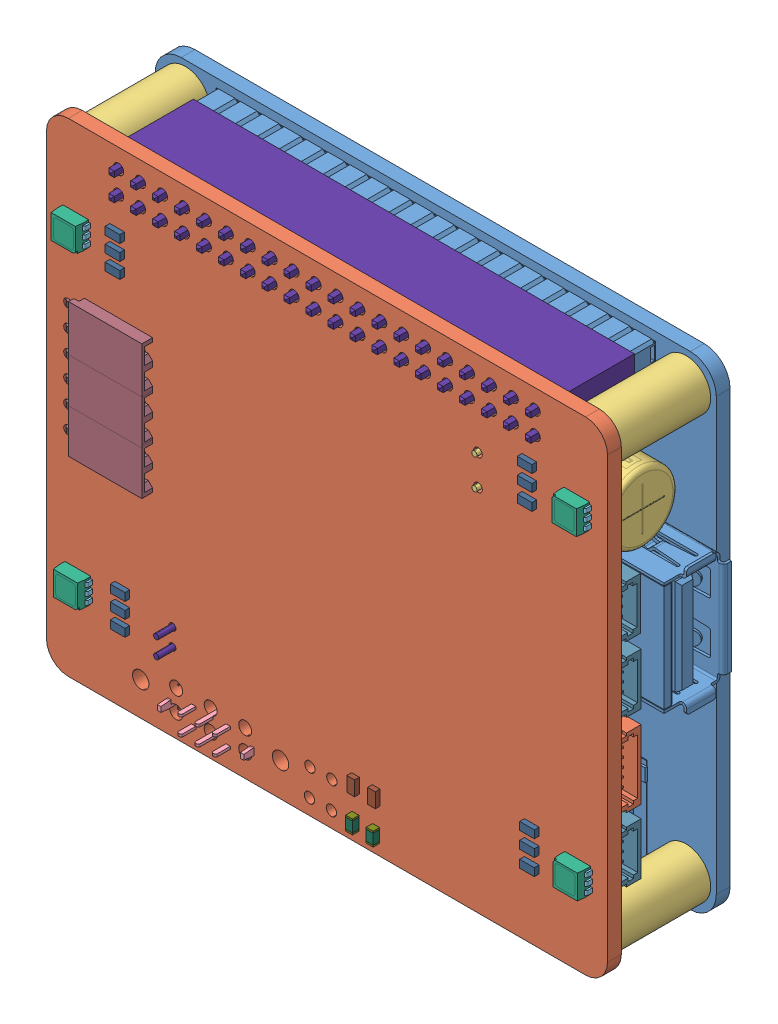
SolidWorks assembly STMf303 hat + RPi 3A+, configuration Default. Lengths in mm.
Overall size (68.17 58.5 17.95).
303 component instances, 40 part files, 5 mates.
Components (placement in the parent):
- Raspberry PI 3 Model A+-1: Raspberry PI 3 Model A+ [Défaut] at (135.3946 10.6154 11.2635) size (68.17 58.5 11.94)
- FC_PiHat_REV1-1: FC_PiHat_REV1 [Default] at (41.2941 -16.4646 23.8635) x (-1 0 0) z (0 0 -1) size (65 56 12.01)
  - FC_PiHat_REV1.step-1: FC_PiHat_REV1.step [Default] at origin size (65 56 12.01)
    - J7FC_PiHat_REV1.step-1: J7FC_PiHat_REV1.step [Default] at origin size (8 4.95 2.96)
      - SM06B-SRSS-TB.step-1: SM06B-SRSS-TB.step [Default] at (13.3 4.6 -0.3) x (1 0 0) z (0 -1 0) size (8 2.96 4.95)
    - C10FC_PiHat_REV1.step-1: C10FC_PiHat_REV1.step [Default] at origin size (13.96 8.06 10.04)
      - User_Library-Cap_electro_8x11_5x3_5mm_RA.step-1: User_Library-Cap_electro_8x11_5x3_5mm_RA.step [Default] at (13.5254 44.5 4) x (0 1 0) z (0 0 1) size (8.06 13.96 10.04)
    - J11FC_PiHat_REV1.step-1: J11FC_PiHat_REV1.step [Default] at origin size (10 6 9.8)
      - User_Library-EG1940-ND.step-1: User_Library-EG1940-ND.step [Default] at (40.9499 0.2249 0) x (1 0 0) z (0 0 1) size (10 6 9.8)
    - D4FC_PiHat_REV1.step-1: D4FC_PiHat_REV1.step [Default] at origin size (3.4 2.8 1.85)
      - User_Library-RGB_LED_Zwart_ASMT-YTC2-0AA02.step-1: User_Library-RGB_LED_Zwart_ASMT-YTC2-0AA02.step [Default] at (2.2908 8.9737 -1.6023) x (-1 0 0) z (0 -1 0) size (3.4 1.85 2.8)
        - Pootje_RGB_LED.step-1: Pootje_RGB_LED.step [Default] at (-0.3594 -0.1975 0.3238) size (0.9 1.1 0.5)
        - ASMT-YTC2-0AA02.step-1: ASMT-YTC2-0AA02.step [Default] at (-2.6594 -0.3475 0.5738) size (3 1.8 2.8)
        - Pootje_RGB_LED.step-2: Pootje_RGB_LED.step [Default] at (-0.3594 -0.1975 -0.5762) size (0.9 1.1 0.5)
        - Pootje_RGB_LED.step-3: Pootje_RGB_LED.step [Default] at (-0.3594 -0.1975 -1.4762) size (0.9 1.1 0.5)
        - Pootje_RGB_LED.step-4: Pootje_RGB_LED.step [Default] at (-1.9594 -0.1975 -1.9762) x (-1 0 0) z (0 0 -1) size (0.9 1.1 0.5)
        - Pootje_RGB_LED.step-5: Pootje_RGB_LED.step [Default] at (-1.9594 -0.1975 -1.0762) x (-1 0 0) z (0 0 -1) size (0.9 1.1 0.5)
        - Pootje_RGB_LED.step-6: Pootje_RGB_LED.step [Default] at (-1.9594 -0.1975 -0.1762) x (-1 0 0) z (0 0 -1) size (0.9 1.1 0.5)
    - D3FC_PiHat_REV1.step-1: D3FC_PiHat_REV1.step [Default] at origin size (3.4 2.8 1.85)
      - User_Library-RGB_LED_Zwart_ASMT-YTC2-0AA02.step-1: User_Library-RGB_LED_Zwart_ASMT-YTC2-0AA02.step [Default] at (2.3908 45.4737 -1.6023) x (-1 0 0) z (0 -1 0) size (3.4 1.85 2.8)
        - Pootje_RGB_LED.step-1: Pootje_RGB_LED.step [Default] at (-0.3594 -0.1975 0.3238) size (0.9 1.1 0.5)
        - ASMT-YTC2-0AA02.step-1: ASMT-YTC2-0AA02.step [Default] at (-2.6594 -0.3475 0.5738) size (3 1.8 2.8)
        - Pootje_RGB_LED.step-2: Pootje_RGB_LED.step [Default] at (-0.3594 -0.1975 -0.5762) size (0.9 1.1 0.5)
        - Pootje_RGB_LED.step-3: Pootje_RGB_LED.step [Default] at (-0.3594 -0.1975 -1.4762) size (0.9 1.1 0.5)
        - Pootje_RGB_LED.step-4: Pootje_RGB_LED.step [Default] at (-1.9594 -0.1975 -1.9762) x (-1 0 0) z (0 0 -1) size (0.9 1.1 0.5)
        - Pootje_RGB_LED.step-5: Pootje_RGB_LED.step [Default] at (-1.9594 -0.1975 -1.0762) x (-1 0 0) z (0 0 -1) size (0.9 1.1 0.5)
        - Pootje_RGB_LED.step-6: Pootje_RGB_LED.step [Default] at (-1.9594 -0.1975 -0.1762) x (-1 0 0) z (0 0 -1) size (0.9 1.1 0.5)
    - D2FC_PiHat_REV1.step-1: D2FC_PiHat_REV1.step [Default] at origin size (3.4 2.8 1.85)
      - User_Library-RGB_LED_Zwart_ASMT-YTC2-0AA02.step-1: User_Library-RGB_LED_Zwart_ASMT-YTC2-0AA02.step [Default] at (62.5092 10.7763 -1.6023) x (1 0 0) z (0 1 0) size (3.4 1.85 2.8)
        - Pootje_RGB_LED.step-1: Pootje_RGB_LED.step [Default] at (-0.3594 -0.1975 0.3238) size (0.9 1.1 0.5)
        - ASMT-YTC2-0AA02.step-1: ASMT-YTC2-0AA02.step [Default] at (-2.6594 -0.3475 0.5738) size (3 1.8 2.8)
        - Pootje_RGB_LED.step-2: Pootje_RGB_LED.step [Default] at (-0.3594 -0.1975 -0.5762) size (0.9 1.1 0.5)
        - Pootje_RGB_LED.step-3: Pootje_RGB_LED.step [Default] at (-0.3594 -0.1975 -1.4762) size (0.9 1.1 0.5)
        - Pootje_RGB_LED.step-4: Pootje_RGB_LED.step [Default] at (-1.9594 -0.1975 -1.9762) x (-1 0 0) z (0 0 -1) size (0.9 1.1 0.5)
        - Pootje_RGB_LED.step-5: Pootje_RGB_LED.step [Default] at (-1.9594 -0.1975 -1.0762) x (-1 0 0) z (0 0 -1) size (0.9 1.1 0.5)
        - Pootje_RGB_LED.step-6: Pootje_RGB_LED.step [Default] at (-1.9594 -0.1975 -0.1762) x (-1 0 0) z (0 0 -1) size (0.9 1.1 0.5)
    - D1FC_PiHat_REV1.step-1: D1FC_PiHat_REV1.step [Default] at origin size (3.4 2.8 1.85)
      - User_Library-RGB_LED_Zwart_ASMT-YTC2-0AA02.step-1: User_Library-RGB_LED_Zwart_ASMT-YTC2-0AA02.step [Default] at (62.7592 46.4263 -1.6023) x (1 0 0) z (0 1 0) size (3.4 1.85 2.8)
        - Pootje_RGB_LED.step-1: Pootje_RGB_LED.step [Default] at (-0.3594 -0.1975 0.3238) size (0.9 1.1 0.5)
        - ASMT-YTC2-0AA02.step-1: ASMT-YTC2-0AA02.step [Default] at (-2.6594 -0.3475 0.5738) size (3 1.8 2.8)
        - Pootje_RGB_LED.step-2: Pootje_RGB_LED.step [Default] at (-0.3594 -0.1975 -0.5762) size (0.9 1.1 0.5)
        - Pootje_RGB_LED.step-3: Pootje_RGB_LED.step [Default] at (-0.3594 -0.1975 -1.4762) size (0.9 1.1 0.5)
        - Pootje_RGB_LED.step-4: Pootje_RGB_LED.step [Default] at (-1.9594 -0.1975 -1.9762) x (-1 0 0) z (0 0 -1) size (0.9 1.1 0.5)
        - Pootje_RGB_LED.step-5: Pootje_RGB_LED.step [Default] at (-1.9594 -0.1975 -1.0762) x (-1 0 0) z (0 0 -1) size (0.9 1.1 0.5)
        - Pootje_RGB_LED.step-6: Pootje_RGB_LED.step [Default] at (-1.9594 -0.1975 -0.1762) x (-1 0 0) z (0 0 -1) size (0.9 1.1 0.5)
    - S1FC_PiHat_REV1.step-1: S1FC_PiHat_REV1.step [Default] at origin size (4.1 4.1 0.81)
      - 5843174976.step-1: 5843174976.step [Default] at (40.7 32.3 0) size (4.1 4.1 0.81)
        - Body.step-1: Body.step [Default] at (-2.05 -2.05 0)
          - Open_CASCADE_STEP_translator_6.8_14.2.1.x_t-1: Open_CASCADE_STEP_translator_6.8_14.2.1.x_t [Default] at origin
        - Open_CASCADE_STEP_translator_6.8_14.1.step-1: Open_CASCADE_STEP_translator_6.8_14.1.step [Default] at (-2.05 -2.05 0) size (0.52 0.52 0.01)
        - Thermal_Shape.step-1: Thermal_Shape.step [Default] at (-1.3 -1.35 -0.001) size (2.6 2.7 0)
        - Pin_Shape.step-1: Pin_Shape.step [Default] at (-2.05 -1.37 0) size (0.35 0.24 0)
        - Pin_Shape.step-2: Pin_Shape.step [Default] at (2.05 1.37 0) x (-1 0 0) z (0 0 1) size (0.35 0.24 0)
        - Pin_Shape.step-3: Pin_Shape.step [Default] at (-2.05 -0.87 0) size (0.35 0.24 0)
        - Pin_Shape.step-4: Pin_Shape.step [Default] at (2.05 0.87 0) x (-1 0 0) z (0 0 1) size (0.35 0.24 0)
        - Pin_Shape.step-5: Pin_Shape.step [Default] at (-2.05 -0.37 0) size (0.35 0.24 0)
        - Pin_Shape.step-6: Pin_Shape.step [Default] at (2.05 0.37 0) x (-1 0 0) z (0 0 1) size (0.35 0.24 0)
        - Pin_Shape.step-7: Pin_Shape.step [Default] at (-2.05 0.13 0) size (0.35 0.24 0)
        - Pin_Shape.step-8: Pin_Shape.step [Default] at (2.05 -0.13 0) x (-1 0 0) z (0 0 1) size (0.35 0.24 0)
        - Pin_Shape.step-9: Pin_Shape.step [Default] at (-2.05 0.63 0) size (0.35 0.24 0)
        - Pin_Shape.step-10: Pin_Shape.step [Default] at (2.05 -0.63 0) x (-1 0 0) z (0 0 1) size (0.35 0.24 0)
        - Pin_Shape.step-11: Pin_Shape.step [Default] at (-2.05 1.13 0) size (0.35 0.24 0)
        - Pin_Shape.step-12: Pin_Shape.step [Default] at (2.05 -1.13 0) x (-1 0 0) z (0 0 1) size (0.35 0.24 0)
        - Pin_Shape.step-13: Pin_Shape.step [Default] at (-1.13 -2.05 0) x (0 1 0) z (0 0 1) size (0.35 0.24 0)
        - Pin_Shape.step-14: Pin_Shape.step [Default] at (1.13 2.05 0) x (0 -1 0) z (0 0 1) size (0.35 0.24 0)
        - Pin_Shape.step-15: Pin_Shape.step [Default] at (-0.63 -2.05 0) x (0 1 0) z (0 0 1) size (0.35 0.24 0)
        - Pin_Shape.step-16: Pin_Shape.step [Default] at (0.63 2.05 0) x (0 -1 0) z (0 0 1) size (0.35 0.24 0)
        - Pin_Shape.step-17: Pin_Shape.step [Default] at (-0.13 -2.05 0) x (0 1 0) z (0 0 1) size (0.35 0.24 0)
        - Pin_Shape.step-18: Pin_Shape.step [Default] at (0.13 2.05 0) x (0 -1 0) z (0 0 1) size (0.35 0.24 0)
        - Pin_Shape.step-19: Pin_Shape.step [Default] at (0.37 -2.05 0) x (0 1 0) z (0 0 1) size (0.35 0.24 0)
        - Pin_Shape.step-20: Pin_Shape.step [Default] at (-0.37 2.05 0) x (0 -1 0) z (0 0 1) size (0.35 0.24 0)
        - Pin_Shape.step-21: Pin_Shape.step [Default] at (0.87 -2.05 0) x (0 1 0) z (0 0 1) size (0.35 0.24 0)
        - Pin_Shape.step-22: Pin_Shape.step [Default] at (-0.87 2.05 0) x (0 -1 0) z (0 0 1) size (0.35 0.24 0)
        - Pin_Shape.step-23: Pin_Shape.step [Default] at (1.37 -2.05 0) x (0 1 0) z (0 0 1) size (0.35 0.24 0)
        - Pin_Shape.step-24: Pin_Shape.step [Default] at (-1.37 2.05 0) x (0 -1 0) z (0 0 1) size (0.35 0.24 0)
    - R14FC_PiHat_REV1.step-1: R14FC_PiHat_REV1.step [Default] at origin size (1.7 0.9 0.55)
      - 6063442624.step-1: 6063442624.step [Default] at (8.7742 7.9 -2.1523) size (1.7 0.9 0.55)
        - Extruded.step-1: Extruded.step [Default] at origin size (1.7 0.9 0.55)
    - R13FC_PiHat_REV1.step-1: R13FC_PiHat_REV1.step [Default] at origin size (1.7 0.9 0.55)
      - 6063442624.step-1: 6063442624.step [Default] at (8.7742 9.8048 -2.1523) size (1.7 0.9 0.55)
        - Extruded.step-1: Extruded.step [Default] at origin size (1.7 0.9 0.55)
    - R12FC_PiHat_REV1.step-1: R12FC_PiHat_REV1.step [Default] at origin size (1.7 0.9 0.55)
      - 6063442624.step-1: 6063442624.step [Default] at (8.7742 11.7 -2.1523) size (1.7 0.9 0.55)
        - Extruded.step-1: Extruded.step [Default] at origin size (1.7 0.9 0.55)
    - R11FC_PiHat_REV1.step-1: R11FC_PiHat_REV1.step [Default] at origin size (1.7 0.9 0.55)
      - 6063442624.step-1: 6063442624.step [Default] at (9.05 44.4 -2.1523) size (1.7 0.9 0.55)
        - Extruded.step-1: Extruded.step [Default] at origin size (1.7 0.9 0.55)
    - R10FC_PiHat_REV1.step-1: R10FC_PiHat_REV1.step [Default] at origin size (1.7 0.9 0.55)
      - 6063442624.step-1: 6063442624.step [Default] at (9.05 46.3 -2.1523) size (1.7 0.9 0.55)
        - Extruded.step-1: Extruded.step [Default] at origin size (1.7 0.9 0.55)
    - R9FC_PiHat_REV1.step-1: R9FC_PiHat_REV1.step [Default] at origin size (0.9 1.7 0.55)
      - 6063442432.step-1: 6063442432.step [Default] at (59.9 29.7 0) size (0.9 1.7 0.55)
        - Extruded-0.step-1: Extruded-0.step [Default] at origin size (0.9 1.7 0.55)
    - R8FC_PiHat_REV1.step-1: R8FC_PiHat_REV1.step [Default] at origin size (1.7 0.9 0.55)
      - 6063442624.step-1: 6063442624.step [Default] at (9.05 48.2 -2.1523) size (1.7 0.9 0.55)
        - Extruded.step-1: Extruded.step [Default] at origin size (1.7 0.9 0.55)
    - R7FC_PiHat_REV1.step-1: R7FC_PiHat_REV1.step [Default] at origin size (1.84 1.84 0.55)
      - 6063441088.step-1: 6063441088.step [Default] at (39.9 37.9 0) size (1.84 1.84 0.55)
        - Extruded-1.step-1: Extruded-1.step [Default] at origin size (1.84 1.84 0.55)
    - R6FC_PiHat_REV1.step-1: R6FC_PiHat_REV1.step [Default] at origin size (1.7 0.9 0.55)
      - 6063442624.step-1: 6063442624.step [Default] at (56.2 11.8 -2.1523) size (1.7 0.9 0.55)
        - Extruded.step-1: Extruded.step [Default] at origin size (1.7 0.9 0.55)
    - R5FC_PiHat_REV1.step-1: R5FC_PiHat_REV1.step [Default] at origin size (1.7 0.9 0.55)
      - 6063442624.step-1: 6063442624.step [Default] at (56.2 10 -2.1523) size (1.7 0.9 0.55)
        - Extruded.step-1: Extruded.step [Default] at origin size (1.7 0.9 0.55)
    - R4FC_PiHat_REV1.step-1: R4FC_PiHat_REV1.step [Default] at origin size (1.7 0.9 0.55)
      - 6063442624.step-1: 6063442624.step [Default] at (56.2 8.2 -2.1523) size (1.7 0.9 0.55)
        - Extruded.step-1: Extruded.step [Default] at origin size (1.7 0.9 0.55)
    - R3FC_PiHat_REV1.step-1: R3FC_PiHat_REV1.step [Default] at origin size (1.7 0.9 0.55)
      - 6063442624.step-1: 6063442624.step [Default] at (56.8 47.4 -2.1523) size (1.7 0.9 0.55)
        - Extruded.step-1: Extruded.step [Default] at origin size (1.7 0.9 0.55)
    - R2FC_PiHat_REV1.step-1: R2FC_PiHat_REV1.step [Default] at origin size (1.7 0.9 0.55)
      - 6063442624.step-1: 6063442624.step [Default] at (56.8 45.6 -2.1523) size (1.7 0.9 0.55)
        - Extruded.step-1: Extruded.step [Default] at origin size (1.7 0.9 0.55)
    - R1FC_PiHat_REV1.step-1: R1FC_PiHat_REV1.step [Default] at origin size (1.7 0.9 0.55)
      - 6063442624.step-1: 6063442624.step [Default] at (56.8 43.8 -2.1523) size (1.7 0.9 0.55)
        - Extruded.step-1: Extruded.step [Default] at origin size (1.7 0.9 0.55)
    - J8FC_PiHat_REV1.step-1: J8FC_PiHat_REV1.step [Default] at origin size (4.95 8 2.96)
      - SM06B-SRSS-TB.step-1: SM06B-SRSS-TB.step [Default] at (4.55 19.8 -0.3) x (0 -1 0) z (-1 0 0) size (8 2.96 4.95)
    - J6FC_PiHat_REV1.step-1: J6FC_PiHat_REV1.step [Default] at origin size (10.06 15.53 5.7)
      - female_header_a-bl254-ea-g02d.step-1: female_header_a-bl254-ea-g02d.step [Default] at (61.2001 31.0851 -1.6023) x (0 -1 0) z (0 0 -1) size (5.33 10.06 5.7)
      - female_header_a-bl254-ea-g02d.step-2: female_header_a-bl254-ea-g02d.step [Default] at (61.2001 26.0099 -1.6023) x (0 -1 0) z (0 0 -1) size (5.33 10.06 5.7)
      - female_header_a-bl254-ea-g02d.step-3: female_header_a-bl254-ea-g02d.step [Default] at (61.2001 36.2099 -1.6023) x (0 -1 0) z (0 0 -1) size (5.33 10.06 5.7)
    - J4FC_PiHat_REV1.step-1: J4FC_PiHat_REV1.step [Default] at origin size (4.95 6 2.96)
      - SM04B-SRSS-TB.step-1: SM04B-SRSS-TB.step [Default] at (4.55 28.375 -0.3) x (0 -1 0) z (-1 0 0) size (6 2.96 4.95)
    - J3FC_PiHat_REV1.step-1: J3FC_PiHat_REV1.step [Default] at origin size (4.95 6 2.96)
      - SM04B-SRSS-TB.step-1: SM04B-SRSS-TB.step [Default] at (4.55 11.35 -0.3) x (0 -1 0) z (-1 0 0) size (6 2.96 4.95)
    - J2FC_PiHat_REV1.step-1: J2FC_PiHat_REV1.step [Default] at origin size (8 4.95 2.96)
      - SM06B-SRSS-TB.step-1: SM06B-SRSS-TB.step [Default] at (22.8093 4.575 -0.3) x (1 0 0) z (0 -1 0) size (8 2.96 4.95)
    - J1FC_PiHat_REV1.step-1: J1FC_PiHat_REV1.step [Default] at origin size (4.95 6 2.96)
      - SM04B-SRSS-TB.step-1: SM04B-SRSS-TB.step [Default] at (4.625 35.925 -0.3) x (0 -1 0) z (-1 0 0) size (6 2.96 4.95)
    - C4FC_PiHat_REV1.step-1: C4FC_PiHat_REV1.step [Default] at origin size (0.9 1.8 0.9)
      - 6063440896.step-1: 6063440896.step [Default] at (41.3 27.825 0) size (0.9 1.8 0.9)
        - Extruded-2.step-1: Extruded-2.step [Default] at origin size (0.9 1.8 0.9)
    - C3FC_PiHat_REV1.step-1: C3FC_PiHat_REV1.step [Default] at origin size (0.9 1.8 0.9)
      - 6063440896.step-1: 6063440896.step [Default] at (44.1 32.225 0) size (0.9 1.8 0.9)
        - Extruded-2.step-1: Extruded-2.step [Default] at origin size (0.9 1.8 0.9)
    - C2FC_PiHat_REV1.step-1: C2FC_PiHat_REV1.step [Default] at origin size (1.8 0.9 0.9)
      - 6063441280.step-1: 6063441280.step [Default] at (38.125 28.8 0) size (1.8 0.9 0.9)
        - Extruded-3.step-1: Extruded-3.step [Default] at origin size (1.8 0.9 0.9)
    - C1FC_PiHat_REV1.step-1: C1FC_PiHat_REV1.step [Default] at origin size (1.8 0.9 0.9)
      - 6063441280.step-1: 6063441280.step [Default] at (38.125 26.7 0) size (1.8 0.9 0.9)
        - Extruded-3.step-1: Extruded-3.step [Default] at origin size (1.8 0.9 0.9)
    - J5FC_PiHat_REV1.step-1: J5FC_PiHat_REV1.step [Default] at origin size (51.1 5 11.1)
      - User_Library-Header_2x20_2_54mm.step-1: User_Library-Header_2x20_2_54mm.step [Default] at (56.6601 52.5601 0) x (1 0 0) z (0 -1 0) size (51.1 11.1 5)
    - L2FC_PiHat_REV1.step-1: L2FC_PiHat_REV1.step [Default] at origin size (12.5 12.7 6.1)
      - 5843174592.step-1: 5843174592.step [Default] at (40.7 17.6 0) x (0 1 0) z (0 0 1) size (12.7 12.5 6.1)
        - pin.step-1: pin.step [Default] at (6.35 2.8 0) x (-1 0 0) z (0 0 1) size (4.5 5.6 3)
          - Open_CASCADE_STEP_translator_6.8_3.3.1.step-1: Open_CASCADE_STEP_translator_6.8_3.3.1.step [Default] at origin size (4.5 5.6 3)
        - pin.step-2: pin.step [Default] at (-6.35 -2.8 0) size (4.5 5.6 3)
          - Open_CASCADE_STEP_translator_6.8_3.3.1.step-1: Open_CASCADE_STEP_translator_6.8_3.3.1.step [Default] at origin size (4.5 5.6 3)
        - Body.step-1: Body.step [Default] at (0 0 0.1)
          - Open_CASCADE_STEP_translator_6.8_14.2.1.x_t-1: Open_CASCADE_STEP_translator_6.8_14.2.1.x_t [Default] at origin
        - cylinder.step-1: cylinder.step [Default] at (0 0 0.1) size (12.5 12.5 3)
    - U3FC_PiHat_REV1.step-1: U3FC_PiHat_REV1.step [Default] at origin size (10.3 15.24 4.47)
      - 5843175168.step-1: 5843175168.step [Default] at (52.775 32.425 0) x (0 1 0) z (0 0 1) size (15.24 10.3 4.47)
        - Body-1.step-1: Body-1.step [Default] at (-4.575 -5.15 0) size (9.15 10.3 4.47)
          - Open_CASCADE_STEP_translator_6.8_42.2.1.step-1: Open_CASCADE_STEP_translator_6.8_42.2.1.step [Default] at origin size (9.15 10.3 4.47)
        - tab.step-1: tab.step [Default] at (-4.575 -5.15 0) size (9 10.25 0.35)
          - Open_CASCADE_STEP_translator_6.8_42.8.1.step-1: Open_CASCADE_STEP_translator_6.8_42.8.1.step [Default] at origin size (9 10.25 0.35)
        - Open_CASCADE_STEP_translator_6.8_42.1.step-1: Open_CASCADE_STEP_translator_6.8_42.1.step [Default] at (-4.575 -5.15 0) size (1.3 1.3 0.01)
        - Lead.step-1: Lead.step [Default] at (-4.575 -3.4 0) x (-1 0 0) z (0 0 1) size (5.46 0.75 2.33)
        - Lead.step-2: Lead.step [Default] at (-4.575 -1.7 0) x (-1 0 0) z (0 0 1) size (5.46 0.75 2.33)
        - Lead.step-3: Lead.step [Default] at (-4.575 0 0) x (-1 0 0) z (0 0 1) size (5.46 0.75 2.33)
        - Lead.step-4: Lead.step [Default] at (-4.575 1.7 0) x (-1 0 0) z (0 0 1) size (5.46 0.75 2.33)
        - Lead.step-5: Lead.step [Default] at (-4.575 3.4 0) x (-1 0 0) z (0 0 1) size (5.46 0.75 2.33)
      - 5843175168-4.step-1: 5843175168-4.step [Default] at (52.775 32.425 0) x (0 1 0) z (0 0 1) size (2.73 0.75 0.2)
    - D6FC_PiHat_REV1.step-1: D6FC_PiHat_REV1.step [Default] at origin size (7.55 6.23 2.62)
      - 5843175552.step-1: 5843175552.step [Default] at (51.8001 16.8001 0) x (1 0 0) z (0 0 1) size (7.55 6.22 2.62)
        - Body-2.step-1: Body-2.step [Default] at (-3.555 -3.11 0.25) size (7.12 6.22 2.47)
          - Open_CASCADE_STEP_translator_6.8_45.1.1.step-1: Open_CASCADE_STEP_translator_6.8_45.1.1.step [Default] at origin size (7.12 6.22 2.47)
        - Lead-5.step-1: Lead-5.step [Default] at (2.635 0 0) size (1.14 3 1.53)
        - Lead-5.step-2: Lead-5.step [Default] at (-2.635 0 0) x (-1 0 0) z (0 0 1) size (1.14 3 1.53)
    - U2FC_PiHat_REV1.step-1: U2FC_PiHat_REV1.step [Default] at origin size (3.98 3.97 1)
      - 5843176128.step-1: 5843176128.step [Default] at (49.3313 45.4354 0) x (0.707107 -0.707107 0) z (0 0 1) size (2.8 2.91 1)
        - Body-3.step-1: Body-3.step [Default] at (-0.8 -1.45 0) size (1.6 2.91 0.95)
          - Open_CASCADE_STEP_translator_6.8_3.1.1.step-1: Open_CASCADE_STEP_translator_6.8_3.1.1.step [Default] at origin size (1.6 2.91 0.95)
        - Leader.step-1: Leader.step [Default] at (-0.8 -0.95 0) x (-1 0 0) z (0 0 1) size (0.6 0.5 0.57)
        - Leader.step-2: Leader.step [Default] at (-0.8 0 0) x (-1 0 0) z (0 0 1) size (0.6 0.5 0.57)
        - Leader.step-3: Leader.step [Default] at (-0.8 0.95 0) x (-1 0 0) z (0 0 1) size (0.6 0.5 0.57)
        - Leader.step-4: Leader.step [Default] at (0.8 -0.95 0) size (0.6 0.5 0.57)
        - Leader.step-5: Leader.step [Default] at (0.8 0.95 0) size (0.6 0.5 0.57)
    - U1FC_PiHat_REV1.step-1: U1FC_PiHat_REV1.step [Default] at origin size (18.98 19.05 1.5)
      - 5843174208.step-1: 5843174208.step [Default] at (26.375 36.65 0) x (-0.707107 -0.707107 0) z (0 0 1) size (14.7 14.7 1.5)
        - Body-4.step-1: Body-4.step [Default] at (-5 -5 0) size (10 10 1.5)
          - Open_CASCADE_STEP_translator_6.8_6.1.1.step-1: Open_CASCADE_STEP_translator_6.8_6.1.1.step [Default] at origin size (10 10 1.5)
        - Leader-6.step-1: Leader-6.step [Default] at (-5 -3.75 0) x (-1 0 0) z (0 0 1) size (2.35 0.27 0.85)
        - Leader-6.step-2: Leader-6.step [Default] at (-3.75 5 0) x (0 1 0) z (0 0 1) size (2.35 0.27 0.85)
        - Leader-6.step-3: Leader-6.step [Default] at (5 -3.75 0) size (2.35 0.27 0.85)
        - Leader-6.step-4: Leader-6.step [Default] at (-3.75 -5 0) x (0 -1 0) z (0 0 1) size (2.35 0.27 0.85)
        - Leader-6.step-5: Leader-6.step [Default] at (-5 -3.25 0) x (-1 0 0) z (0 0 1) size (2.35 0.27 0.85)
        - Leader-6.step-6: Leader-6.step [Default] at (-3.25 5 0) x (0 1 0) z (0 0 1) size (2.35 0.27 0.85)
        - Leader-6.step-7: Leader-6.step [Default] at (5 -3.25 0) size (2.35 0.27 0.85)
        - Leader-6.step-8: Leader-6.step [Default] at (-3.25 -5 0) x (0 -1 0) z (0 0 1) size (2.35 0.27 0.85)
        - Leader-6.step-9: Leader-6.step [Default] at (-5 -2.75 0) x (-1 0 0) z (0 0 1) size (2.35 0.27 0.85)
        - Leader-6.step-10: Leader-6.step [Default] at (-2.75 5 0) x (0 1 0) z (0 0 1) size (2.35 0.27 0.85)
        - Leader-6.step-11: Leader-6.step [Default] at (5 -2.75 0) size (2.35 0.27 0.85)
        - Leader-6.step-12: Leader-6.step [Default] at (-2.75 -5 0) x (0 -1 0) z (0 0 1) size (2.35 0.27 0.85)
        - Leader-6.step-13: Leader-6.step [Default] at (-5 -2.25 0) x (-1 0 0) z (0 0 1) size (2.35 0.27 0.85)
        - Leader-6.step-14: Leader-6.step [Default] at (-2.25 5 0) x (0 1 0) z (0 0 1) size (2.35 0.27 0.85)
        - Leader-6.step-15: Leader-6.step [Default] at (5 -2.25 0) size (2.35 0.27 0.85)
        - Leader-6.step-16: Leader-6.step [Default] at (-2.25 -5 0) x (0 -1 0) z (0 0 1) size (2.35 0.27 0.85)
        - Leader-6.step-17: Leader-6.step [Default] at (-5 -1.75 0) x (-1 0 0) z (0 0 1) size (2.35 0.27 0.85)
        - Leader-6.step-18: Leader-6.step [Default] at (-1.75 5 0) x (0 1 0) z (0 0 1) size (2.35 0.27 0.85)
        - Leader-6.step-19: Leader-6.step [Default] at (5 -1.75 0) size (2.35 0.27 0.85)
        - Leader-6.step-20: Leader-6.step [Default] at (-1.75 -5 0) x (0 -1 0) z (0 0 1) size (2.35 0.27 0.85)
        - Leader-6.step-21: Leader-6.step [Default] at (-5 -1.25 0) x (-1 0 0) z (0 0 1) size (2.35 0.27 0.85)
        - Leader-6.step-22: Leader-6.step [Default] at (-1.25 5 0) x (0 1 0) z (0 0 1) size (2.35 0.27 0.85)
        - Leader-6.step-23: Leader-6.step [Default] at (5 -1.25 0) size (2.35 0.27 0.85)
        - Leader-6.step-24: Leader-6.step [Default] at (-1.25 -5 0) x (0 -1 0) z (0 0 1) size (2.35 0.27 0.85)
        - Leader-6.step-25: Leader-6.step [Default] at (-5 -0.75 0) x (-1 0 0) z (0 0 1) size (2.35 0.27 0.85)
        - Leader-6.step-26: Leader-6.step [Default] at (-0.75 5 0) x (0 1 0) z (0 0 1) size (2.35 0.27 0.85)
        - Leader-6.step-27: Leader-6.step [Default] at (5 -0.75 0) size (2.35 0.27 0.85)
        - Leader-6.step-28: Leader-6.step [Default] at (-0.75 -5 0) x (0 -1 0) z (0 0 1) size (2.35 0.27 0.85)
        - Leader-6.step-29: Leader-6.step [Default] at (-5 -0.25 0) x (-1 0 0) z (0 0 1) size (2.35 0.27 0.85)
        - Leader-6.step-30: Leader-6.step [Default] at (-0.25 5 0) x (0 1 0) z (0 0 1) size (2.35 0.27 0.85)
        - Leader-6.step-31: Leader-6.step [Default] at (5 -0.25 0) size (2.35 0.27 0.85)
        - Leader-6.step-32: Leader-6.step [Default] at (-0.25 -5 0) x (0 -1 0) z (0 0 1) size (2.35 0.27 0.85)
        - Leader-6.step-33: Leader-6.step [Default] at (-5 0.25 0) x (-1 0 0) z (0 0 1) size (2.35 0.27 0.85)
        - Leader-6.step-34: Leader-6.step [Default] at (0.25 5 0) x (0 1 0) z (0 0 1) size (2.35 0.27 0.85)
        - Leader-6.step-35: Leader-6.step [Default] at (5 0.25 0) size (2.35 0.27 0.85)
        - Leader-6.step-36: Leader-6.step [Default] at (0.25 -5 0) x (0 -1 0) z (0 0 1) size (2.35 0.27 0.85)
        - Leader-6.step-37: Leader-6.step [Default] at (-5 0.75 0) x (-1 0 0) z (0 0 1) size (2.35 0.27 0.85)
        - Leader-6.step-38: Leader-6.step [Default] at (0.75 5 0) x (0 1 0) z (0 0 1) size (2.35 0.27 0.85)
        - Leader-6.step-39: Leader-6.step [Default] at (5 0.75 0) size (2.35 0.27 0.85)
        - Leader-6.step-40: Leader-6.step [Default] at (0.75 -5 0) x (0 -1 0) z (0 0 1) size (2.35 0.27 0.85)
        - Leader-6.step-41: Leader-6.step [Default] at (-5 1.25 0) x (-1 0 0) z (0 0 1) size (2.35 0.27 0.85)
        - Leader-6.step-42: Leader-6.step [Default] at (1.25 5 0) x (0 1 0) z (0 0 1) size (2.35 0.27 0.85)
        - Leader-6.step-43: Leader-6.step [Default] at (5 1.25 0) size (2.35 0.27 0.85)
        - Leader-6.step-44: Leader-6.step [Default] at (1.25 -5 0) x (0 -1 0) z (0 0 1) size (2.35 0.27 0.85)
        - Leader-6.step-45: Leader-6.step [Default] at (-5 1.75 0) x (-1 0 0) z (0 0 1) size (2.35 0.27 0.85)
        - Leader-6.step-46: Leader-6.step [Default] at (1.75 5 0) x (0 1 0) z (0 0 1) size (2.35 0.27 0.85)
        - Leader-6.step-47: Leader-6.step [Default] at (5 1.75 0) size (2.35 0.27 0.85)
        - Leader-6.step-48: Leader-6.step [Default] at (1.75 -5 0) x (0 -1 0) z (0 0 1) size (2.35 0.27 0.85)
        - Leader-6.step-49: Leader-6.step [Default] at (-5 2.25 0) x (-1 0 0) z (0 0 1) size (2.35 0.27 0.85)
        - Leader-6.step-50: Leader-6.step [Default] at (2.25 5 0) x (0 1 0) z (0 0 1) size (2.35 0.27 0.85)
        - Leader-6.step-51: Leader-6.step [Default] at (5 2.25 0) size (2.35 0.27 0.85)
        - Leader-6.step-52: Leader-6.step [Default] at (2.25 -5 0) x (0 -1 0) z (0 0 1) size (2.35 0.27 0.85)
        - Leader-6.step-53: Leader-6.step [Default] at (-5 2.75 0) x (-1 0 0) z (0 0 1) size (2.35 0.27 0.85)
        - Leader-6.step-54: Leader-6.step [Default] at (2.75 5 0) x (0 1 0) z (0 0 1) size (2.35 0.27 0.85)
        - Leader-6.step-55: Leader-6.step [Default] at (5 2.75 0) size (2.35 0.27 0.85)
        - Leader-6.step-56: Leader-6.step [Default] at (2.75 -5 0) x (0 -1 0) z (0 0 1) size (2.35 0.27 0.85)
        - Leader-6.step-57: Leader-6.step [Default] at (-5 3.25 0) x (-1 0 0) z (0 0 1) size (2.35 0.27 0.85)
        - Leader-6.step-58: Leader-6.step [Default] at (3.25 5 0) x (0 1 0) z (0 0 1) size (2.35 0.27 0.85)
        - Leader-6.step-59: Leader-6.step [Default] at (5 3.25 0) size (2.35 0.27 0.85)
        - Leader-6.step-60: Leader-6.step [Default] at (3.25 -5 0) x (0 -1 0) z (0 0 1) size (2.35 0.27 0.85)
        - Leader-6.step-61: Leader-6.step [Default] at (-5 3.75 0) x (-1 0 0) z (0 0 1) size (2.35 0.27 0.85)
        - Leader-6.step-62: Leader-6.step [Default] at (3.75 5 0) x (0 1 0) z (0 0 1) size (2.35 0.27 0.85)
        - Leader-6.step-63: Leader-6.step [Default] at (5 3.75 0) size (2.35 0.27 0.85)
        - Leader-6.step-64: Leader-6.step [Default] at (3.75 -5 0) x (0 -1 0) z (0 0 1) size (2.35 0.27 0.85)
    - R17FC_PiHat_REV1.step-1: R17FC_PiHat_REV1.step [Default] at origin size (0.9 1.7 0.55)
      - 6063442432.step-1: 6063442432.step [Default] at (29.2 5.9 -2.1523) size (0.9 1.7 0.55)
        - Extruded-0.step-1: Extruded-0.step [Default] at origin size (0.9 1.7 0.55)
    - R15FC_PiHat_REV1.step-1: R15FC_PiHat_REV1.step [Default] at origin size (0.9 1.7 0.55)
      - 6063442432.step-1: 6063442432.step [Default] at (26.8 5.9 -2.1523) size (0.9 1.7 0.55)
        - Extruded-0.step-1: Extruded-0.step [Default] at origin size (0.9 1.7 0.55)
    - Q1FC_PiHat_REV1.step-1: Q1FC_PiHat_REV1.step [Default] at origin size (3.2 5 1.35)
      - User_Library-445-CRYTAL-SMD.step-1: User_Library-445-CRYTAL-SMD.step [Default] at (37.4671 49.9363 0.0126) x (0 1 0) z (1 0 0) size (5 1.35 3.2)
    - L3FC_PiHat_REV1.step-1: L3FC_PiHat_REV1.step [Default] at origin size (12.5 12.7 6.1)
      - 5843174592.step-1: 5843174592.step [Default] at (27.5 17.6 0) x (0 1 0) z (0 0 1) size (12.7 12.5 6.1)
        - pin.step-1: pin.step [Default] at (6.35 2.8 0) x (-1 0 0) z (0 0 1) size (4.5 5.6 3)
          - Open_CASCADE_STEP_translator_6.8_3.3.1.step-1: Open_CASCADE_STEP_translator_6.8_3.3.1.step [Default] at origin size (4.5 5.6 3)
        - pin.step-2: pin.step [Default] at (-6.35 -2.8 0) size (4.5 5.6 3)
          - Open_CASCADE_STEP_translator_6.8_3.3.1.step-1: Open_CASCADE_STEP_translator_6.8_3.3.1.step [Default] at origin size (4.5 5.6 3)
        - Body.step-1: Body.step [Default] at (0 0 0.1)
          - Open_CASCADE_STEP_translator_6.8_14.2.1.x_t-1: Open_CASCADE_STEP_translator_6.8_14.2.1.x_t [Default] at origin
        - cylinder.step-1: cylinder.step [Default] at (0 0 0.1) size (12.5 12.5 3)
    - L1FC_PiHat_REV1.step-1: L1FC_PiHat_REV1.step [Default] at origin size (3.68 3.68 1.5)
      - 6063441856.step-1: 6063441856.step [Default] at (51.5 42 0) size (3.68 3.68 1.5)
        - Extruded-7.step-1: Extruded-7.step [Default] at origin size (3.68 3.68 1.5)
    - D7FC_PiHat_REV1.step-1: D7FC_PiHat_REV1.step [Default] at origin size (0.8 1.6 0.75)
      - 6063441664.step-1: 6063441664.step [Default] at (29.2 2.1 -2.3523) size (0.8 1.2 0.75)
        - Extruded-8.step-1: Extruded-8.step [Default] at origin size (0.8 1.2 0.75)
      - 6063441472.step-1: 6063441472.step [Default] at (29.2 2.8 -2.3523) size (0.8 0.2 0.75)
        - Extruded-9.step-1: Extruded-9.step [Default] at origin size (0.8 0.2 0.75)
      - 6063441472.step-2: 6063441472.step [Default] at (29.2 1.4 -2.3523) size (0.8 0.2 0.75)
        - Extruded-9.step-1: Extruded-9.step [Default] at origin size (0.8 0.2 0.75)
    - D5FC_PiHat_REV1.step-1: D5FC_PiHat_REV1.step [Default] at origin size (0.8 1.6 0.75)
      - 6063441664.step-1: 6063441664.step [Default] at (26.8 2.075 -2.3523) size (0.8 1.2 0.75)
        - Extruded-8.step-1: Extruded-8.step [Default] at origin size (0.8 1.2 0.75)
      - 6063441472.step-1: 6063441472.step [Default] at (26.8 2.775 -2.3523) size (0.8 0.2 0.75)
        - Extruded-9.step-1: Extruded-9.step [Default] at origin size (0.8 0.2 0.75)
      - 6063441472.step-2: 6063441472.step [Default] at (26.8 1.375 -2.3523) size (0.8 0.2 0.75)
        - Extruded-9.step-1: Extruded-9.step [Default] at origin size (0.8 0.2 0.75)
    - C9FC_PiHat_REV1.step-1: C9FC_PiHat_REV1.step [Default] at origin size (13.46 5.06 8.54)
      - User_Library-Cap_electro_5x11x2mm_RA.step-1: User_Library-Cap_electro_5x11x2mm_RA.step [Default] at (51.885 9.9755 2.5) x (0 -1 0) z (0 0 1) size (5.06 13.46 8.54)
    - C8FC_PiHat_REV1.step-1: C8FC_PiHat_REV1.step [Default] at origin size (1.91 1.91 0.9)
      - 6063442048.step-1: 6063442048.step [Default] at (47.1 43.3857 0) size (1.91 1.91 0.9)
        - Extruded-10.step-1: Extruded-10.step [Default] at origin size (1.91 1.91 0.9)
    - C7FC_PiHat_REV1.step-1: C7FC_PiHat_REV1.step [Default] at origin size (1.91 1.91 0.9)
      - 6063442240.step-1: 6063442240.step [Default] at (45.7 46.4 0) size (1.91 1.91 0.9)
        - Extruded-11.step-1: Extruded-11.step [Default] at origin size (1.91 1.91 0.9)
    - C6FC_PiHat_REV1.step-1: C6FC_PiHat_REV1.step [Default] at origin size (1.8 0.9 0.9)
      - 6063441280.step-1: 6063441280.step [Default] at (39.9535 42.2416 0) size (1.8 0.9 0.9)
        - Extruded-3.step-1: Extruded-3.step [Default] at origin size (1.8 0.9 0.9)
    - C5FC_PiHat_REV1.step-1: C5FC_PiHat_REV1.step [Default] at origin size (1.8 0.9 0.9)
      - 6063441280.step-1: 6063441280.step [Default] at (39.9535 44.9915 0) size (1.8 0.9 0.9)
        - Extruded-3.step-1: Extruded-3.step [Default] at origin size (1.8 0.9 0.9)
    - BoardFC_PiHat_REV1.step-1: BoardFC_PiHat_REV1.step [Default] at origin size (65 56 1.6)
- Spacer-1: Spacer [Default] at (37.7941 -12.9363 12.8635) x (-1 0 0) z (0 1 0) size (5.7 11 5.7)
- Spacer-2: Spacer [Default] at (-20.2059 -12.9363 12.8635) x (1 0 0) z (0 -1 0) size (5.7 11 5.7)
- Spacer-3: Spacer [Default] at (-20.2059 36.0637 12.8635) x (1 0 0) z (0 -1 0) size (5.7 11 5.7)
- Spacer-4: Spacer [Default] at (37.7941 36.0637 12.8635) x (-1 0 0) z (0 1 0) size (5.7 11 5.7)
Mates (geometry in assembly coordinates):
- Coincident1: coincident anti-aligned: plane of Raspberry PI 3 Model A+-1 through (-15.4142 35.0854 15.3635) normal (0 0 1); plane of FC_PiHat_REV1-1/FC_PiHat_REV1.step-1/J5FC_PiHat_REV1.step-1/User_Library-Header_2x20_2_54mm.step-1 through (-13.946 33.5954 15.3635) normal (0 0 -1)
- Coincident2: coincident aligned: plane of Raspberry PI 3 Model A+-1 through (-23.7059 11.5637 12.8635) normal (-1 0 0); plane of FC_PiHat_REV1-1/FC_PiHat_REV1.step-1/BoardFC_PiHat_REV1.step-1 through (-23.7059 36.9954 25.4659) normal (-1 0 0)
- Coincident10: coincident: plane of Raspberry PI 3 Model A+-1 through (33.8158 38.5954 12.8635) normal (0 1 0); line of FC_PiHat_REV1-1/FC_PiHat_REV1.step-1/J5FC_PiHat_REV1.step-1/User_Library-Header_2x20_2_54mm.step-1 through (34.314 38.5954 23.8635) axis (0 0 -1)
- Coincident11: coincident anti-aligned: plane of Raspberry PI 3 Model A+-1 through (18.7941 11.5637 12.8635) normal (0 0 1); plane of Spacer-1 through (37.7941 -12.9363 12.8635) normal (0 0 -1)
- Concentric1: concentric anti-aligned: cylinder of Raspberry PI 3 Model A+-1 through (37.7941 -12.9363 12.8635) axis (0 0 -1) radius 1.375; circle of Spacer-1
